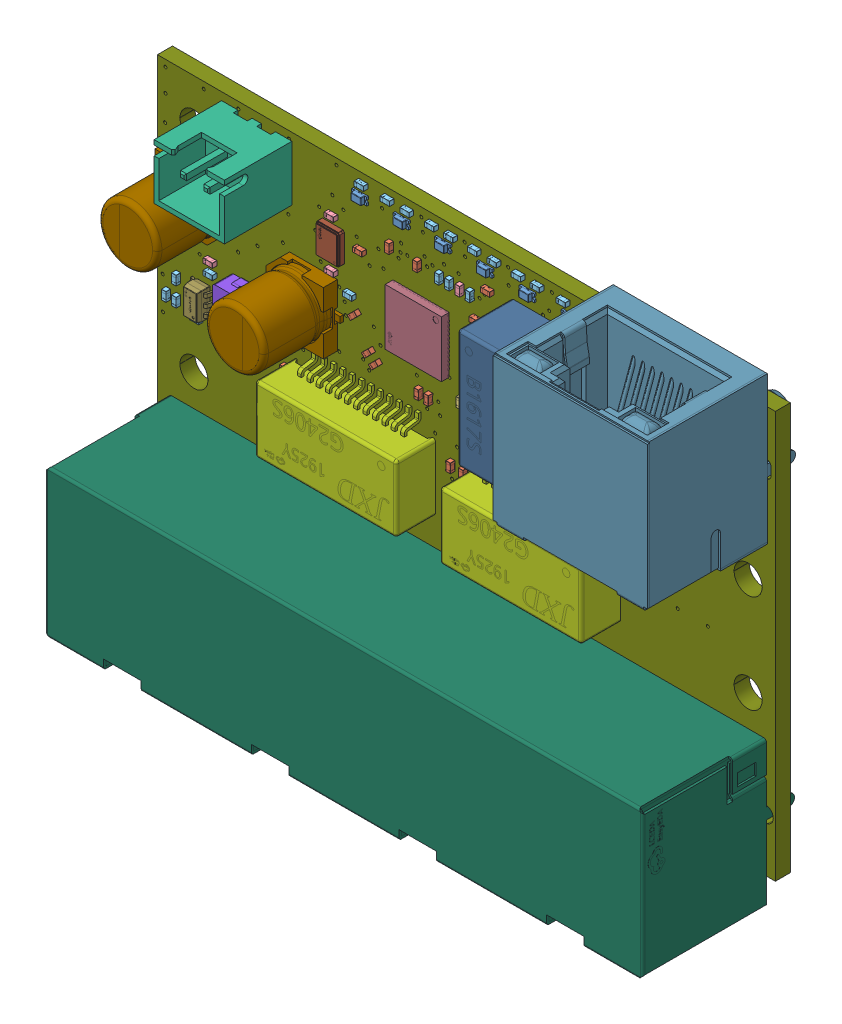
SolidWorks assembly 交换机, configuration 默认. Lengths in mm.
Overall size (65.92 49.68 16.5).
179 component instances, 16 part files, 0 mates.
Components (placement in the parent):
- LX-SWF502-2.step-1: LX-SWF502-2.step [Default] at (-129.5338 -11.9883 -6.5513) size (65.92 49.68 16.5)
  - RJEO-D19.step-1: RJEO-D19.step [Default] at (21.7657 41.0001 1.6) size (1.62 0.82 0.56)
    - LED0603N.step-1: LED0603N.step [Default] at origin size (1.62 0.82 0.56)
      - COMPOUND.step-1: COMPOUND.step [Default] at origin size (1.62 0.82 0.56)
  - RJEO-D2.step-1: RJEO-D2.step [Default] at (30.6411 41.0001 1.6) size (1.62 0.82 0.56)
    - LED0603N.step-1: LED0603N.step [Default] at origin size (1.62 0.82 0.56)
      - COMPOUND.step-1: COMPOUND.step [Default] at origin size (1.62 0.82 0.56)
  - RJEO-D20.step-1: RJEO-D20.step [Default] at (44.1334 41.0001 1.6) size (1.62 0.82 0.56)
    - LED0603N.step-1: LED0603N.step [Default] at origin size (1.62 0.82 0.56)
      - COMPOUND.step-1: COMPOUND.step [Default] at origin size (1.62 0.82 0.56)
  - RJEO-D21.step-1: RJEO-D21.step [Default] at (39.6501 41.0001 1.6) size (1.62 0.82 0.56)
    - LED0603N.step-1: LED0603N.step [Default] at origin size (1.62 0.82 0.56)
      - COMPOUND.step-1: COMPOUND.step [Default] at origin size (1.62 0.82 0.56)
  - RJEO-D22.step-1: RJEO-D22.step [Default] at (35.1271 41.0001 1.6) size (1.62 0.82 0.56)
    - LED0603N.step-1: LED0603N.step [Default] at origin size (1.62 0.82 0.56)
      - COMPOUND.step-1: COMPOUND.step [Default] at origin size (1.62 0.82 0.56)
  - RJEO-D1.step-1: RJEO-D1.step [Default] at (26.2147 41.0001 1.6) size (1.62 0.82 0.56)
    - LED0603N.step-1: LED0603N.step [Default] at origin size (1.62 0.82 0.56)
      - COMPOUND.step-1: COMPOUND.step [Default] at origin size (1.62 0.82 0.56)
  - RJEO-C10.step-1: RJEO-C10.step [Default] at (28.0001 37.4021 1.6) x (0 1 0) z (0 0 1) size (1 0.5 0.5)
    - 0402.step-1: 0402.step [Default] at origin size (1 0.5 0.5)
      - SOLID.step-1: SOLID.step [Default] at origin size (1 0.5 0.5)
  - RJEO-C11.step-1: RJEO-C11.step [Default] at (22.346 36.1431 1.6) x (-1 0 0) z (0 0 1) size (1 0.5 0.5)
    - 0402.step-1: 0402.step [Default] at origin size (1 0.5 0.5)
      - SOLID.step-1: SOLID.step [Default] at origin size (1 0.5 0.5)
  - RJEO-C13.step-1: RJEO-C13.step [Default] at (28.1391 26.6451 1.6) x (0 -1 0) z (0 0 1) size (1 0.5 0.5)
    - 0402.step-1: 0402.step [Default] at origin size (1 0.5 0.5)
      - SOLID.step-1: SOLID.step [Default] at origin size (1 0.5 0.5)
  - RJEO-C14.step-1: RJEO-C14.step [Default] at (32.6271 28.0611 1.6) x (0 -1 0) z (0 0 1) size (1 0.5 0.5)
    - 0402-1.step-1: 0402-1.step [Default] at origin size (1 0.5 0.5)
      - SOLID-0.step-1: SOLID-0.step [Default] at origin size (1 0.5 0.5)
  - RJEO-C15.step-1: RJEO-C15.step [Default] at (33.7611 35.9131 1.6) size (1 0.5 0.5)
    - 0402.step-1: 0402.step [Default] at origin size (1 0.5 0.5)
      - SOLID.step-1: SOLID.step [Default] at origin size (1 0.5 0.5)
  - RJEO-C16.step-1: RJEO-C16.step [Default] at (25.0001 37.5751 1.6) x (0 1 0) z (0 0 1) size (1 0.5 0.5)
    - 0402.step-1: 0402.step [Default] at origin size (1 0.5 0.5)
      - SOLID.step-1: SOLID.step [Default] at origin size (1 0.5 0.5)
  - RJEO-C17.step-1: RJEO-C17.step [Default] at (21.666 30.3191 1.6) x (-0.707107 -0.707107 0) z (0 0 1) size (1 0.5 0.5)
    - 0402.step-1: 0402.step [Default] at origin size (1 0.5 0.5)
      - SOLID.step-1: SOLID.step [Default] at origin size (1 0.5 0.5)
  - RJEO-C18.step-1: RJEO-C18.step [Default] at (23.917 26.8671 1.6) x (-0.707107 -0.707107 0) z (0 0 1) size (1 0.5 0.5)
    - 0402.step-1: 0402.step [Default] at origin size (1 0.5 0.5)
      - SOLID.step-1: SOLID.step [Default] at origin size (1 0.5 0.5)
  - RJEO-C19.step-1: RJEO-C19.step [Default] at (34.9891 39.2441 1.6) size (1 0.5 0.5)
    - 0402.step-1: 0402.step [Default] at origin size (1 0.5 0.5)
      - SOLID.step-1: SOLID.step [Default] at origin size (1 0.5 0.5)
  - RJEO-C2.step-1: RJEO-C2.step [Default] at (32.8971 20.6 1.6) x (0 1 0) z (0 0 1) size (1 0.5 0.5)
    - 0402.step-1: 0402.step [Default] at origin size (1 0.5 0.5)
      - SOLID.step-1: SOLID.step [Default] at origin size (1 0.5 0.5)
  - RJEO-C20.step-1: RJEO-C20.step [Default] at (31.5481 20.6 1.6) x (0 1 0) z (0 0 1) size (1 0.5 0.5)
    - 0402.step-1: 0402.step [Default] at origin size (1 0.5 0.5)
      - SOLID.step-1: SOLID.step [Default] at origin size (1 0.5 0.5)
  - RJEO-C25.step-1: RJEO-C25.step [Default] at (13.815 20.6 1.6) x (0 1 0) z (0 0 1) size (1 0.5 0.5)
    - 0402.step-1: 0402.step [Default] at origin size (1 0.5 0.5)
      - SOLID.step-1: SOLID.step [Default] at origin size (1 0.5 0.5)
  - RJEO-C37.step-1: RJEO-C37.step [Default] at (23.177 27.5921 1.6) x (-0.707107 -0.707107 0) z (0 0 1) size (1 0.5 0.5)
    - 0402.step-1: 0402.step [Default] at origin size (1 0.5 0.5)
      - SOLID.step-1: SOLID.step [Default] at origin size (1 0.5 0.5)
  - RJEO-C7.step-1: RJEO-C7.step [Default] at (34.7321 30.7291 1.6) x (0 -1 0) z (0 0 1) size (1 0.5 0.5)
    - 0402.step-1: 0402.step [Default] at origin size (1 0.5 0.5)
      - SOLID.step-1: SOLID.step [Default] at origin size (1 0.5 0.5)
  - RJEO-C8.step-1: RJEO-C8.step [Default] at (29.1961 26.6451 1.6) x (0 -1 0) z (0 0 1) size (1 0.5 0.5)
    - 0402.step-1: 0402.step [Default] at origin size (1 0.5 0.5)
      - SOLID.step-1: SOLID.step [Default] at origin size (1 0.5 0.5)
  - RJEO-C21.step-1: RJEO-C21.step [Default] at (5.908 27.1321 1.6) x (-1 0 0) z (0 0 1) size (1 0.5 0.5)
    - C0402.step-1: C0402.step [Default] at origin size (1 0.5 0.5)
      - SOLID-1.step-1: SOLID-1.step [Default] at origin size (1 0.5 0.5)
  - RJEO-C22.step-1: RJEO-C22.step [Default] at (6.552 21.19 1.6) size (1 0.5 0.5)
    - C0402.step-1: C0402.step [Default] at origin size (1 0.5 0.5)
      - SOLID-1.step-1: SOLID-1.step [Default] at origin size (1 0.5 0.5)
  - RJEO-C3.step-1: RJEO-C3.step [Default] at (32.5331 37.9101 1.6) x (0 1 0) z (0 0 1) size (1 0.5 0.5)
    - C0402.step-1: C0402.step [Default] at origin size (1 0.5 0.5)
      - SOLID-1.step-1: SOLID-1.step [Default] at origin size (1 0.5 0.5)
  - RJEO-C4.step-1: RJEO-C4.step [Default] at (18.817 32.7271 1.6) x (-1 0 0) z (0 0 1) size (1 0.5 0.5)
    - C0402.step-1: C0402.step [Default] at origin size (1 0.5 0.5)
      - SOLID-1.step-1: SOLID-1.step [Default] at origin size (1 0.5 0.5)
  - RJEO-C5.step-1: RJEO-C5.step [Default] at (18.81 37.8231 1.6) x (-1 0 0) z (0 0 1) size (1 0.5 0.5)
    - C0402.step-1: C0402.step [Default] at origin size (1 0.5 0.5)
      - SOLID-1.step-1: SOLID-1.step [Default] at origin size (1 0.5 0.5)
  - RJEO-C1.step-1: RJEO-C1.step [Default] at (51.3311 20.6 1.6) x (0 1 0) z (0 0 1) size (1 0.5 0.5)
    - 0402.step-1: 0402.step [Default] at origin size (1 0.5 0.5)
      - SOLID.step-1: SOLID.step [Default] at origin size (1 0.5 0.5)
  - RJEO-R11.step-1: RJEO-R11.step [Default] at (6.402 25.9921 1.6) x (-1 0 0) z (0 0 1) size (1 0.5 0.5)
    - 0402-2.step-1: 0402-2.step [Default] at origin size (1 0.5 0.5)
      - SOLID-2.step-1: SOLID-2.step [Default] at origin size (1 0.5 0.5)
  - RJEO-R12.step-1: RJEO-R12.step [Default] at (3.948 21.19 1.6) size (1 0.5 0.5)
    - 0402-2.step-1: 0402-2.step [Default] at origin size (1 0.5 0.5)
      - SOLID-2.step-1: SOLID-2.step [Default] at origin size (1 0.5 0.5)
  - RJEO-R13.step-1: RJEO-R13.step [Default] at (1.211 22.273 1.6) x (0 -1 0) z (0 0 1) size (1 0.5 0.5)
    - 0402-2.step-1: 0402-2.step [Default] at origin size (1 0.5 0.5)
      - SOLID-2.step-1: SOLID-2.step [Default] at origin size (1 0.5 0.5)
  - RJEO-R14.step-1: RJEO-R14.step [Default] at (2.295 24.326 1.6) x (0 -1 0) z (0 0 1) size (1 0.5 0.5)
    - 0402-2.step-1: 0402-2.step [Default] at origin size (1 0.5 0.5)
      - SOLID-2.step-1: SOLID-2.step [Default] at origin size (1 0.5 0.5)
  - RJEO-R15.step-1: RJEO-R15.step [Default] at (2.295 21.285 1.6) x (0 1 0) z (0 0 1) size (1 0.5 0.5)
    - 0402-2.step-1: 0402-2.step [Default] at origin size (1 0.5 0.5)
      - SOLID-2.step-1: SOLID-2.step [Default] at origin size (1 0.5 0.5)
  - RJEO-R2.step-1: RJEO-R2.step [Default] at (20.272 31.5191 1.6) size (1 0.5 0.5)
    - 0402-2.step-1: 0402-2.step [Default] at origin size (1 0.5 0.5)
      - SOLID-2.step-1: SOLID-2.step [Default] at origin size (1 0.5 0.5)
  - RJEO-R20.step-1: RJEO-R20.step [Default] at (26.4001 42.3001 1.6) size (1 0.5 0.5)
    - 0402-2.step-1: 0402-2.step [Default] at origin size (1 0.5 0.5)
      - SOLID-2.step-1: SOLID-2.step [Default] at origin size (1 0.5 0.5)
  - RJEO-R21.step-1: RJEO-R21.step [Default] at (31.0661 42.3001 1.6) size (1 0.5 0.5)
    - 0402-2.step-1: 0402-2.step [Default] at origin size (1 0.5 0.5)
      - SOLID-2.step-1: SOLID-2.step [Default] at origin size (1 0.5 0.5)
  - RJEO-R22.step-1: RJEO-R22.step [Default] at (35.6971 42.3001 1.6) size (1 0.5 0.5)
    - 0402-2.step-1: 0402-2.step [Default] at origin size (1 0.5 0.5)
      - SOLID-2.step-1: SOLID-2.step [Default] at origin size (1 0.5 0.5)
  - RJEO-R23.step-1: RJEO-R23.step [Default] at (40.2871 42.3001 1.6) size (1 0.5 0.5)
    - 0402-2.step-1: 0402-2.step [Default] at origin size (1 0.5 0.5)
      - SOLID-2.step-1: SOLID-2.step [Default] at origin size (1 0.5 0.5)
  - RJEO-R24.step-1: RJEO-R24.step [Default] at (45.0261 42.3001 1.6) size (1 0.5 0.5)
    - 0402-2.step-1: 0402-2.step [Default] at origin size (1 0.5 0.5)
      - SOLID-2.step-1: SOLID-2.step [Default] at origin size (1 0.5 0.5)
  - RJEO-R26.step-1: RJEO-R26.step [Default] at (21.524 42.3001 1.6) size (1 0.5 0.5)
    - 0402-2.step-1: 0402-2.step [Default] at origin size (1 0.5 0.5)
      - SOLID-2.step-1: SOLID-2.step [Default] at origin size (1 0.5 0.5)
  - RJEO-R3.step-1: RJEO-R3.step [Default] at (33.6221 38.4311 1.6) x (0 -1 0) z (0 0 1) size (1 0.5 0.5)
    - 0402-2.step-1: 0402-2.step [Default] at origin size (1 0.5 0.5)
      - SOLID-2.step-1: SOLID-2.step [Default] at origin size (1 0.5 0.5)
  - RJEO-R4.step-1: RJEO-R4.step [Default] at (30.3291 38.4071 1.6) x (0 -1 0) z (0 0 1) size (1 0.5 0.5)
    - 0402-2.step-1: 0402-2.step [Default] at origin size (1 0.5 0.5)
      - SOLID-2.step-1: SOLID-2.step [Default] at origin size (1 0.5 0.5)
  - RJEO-R5.step-1: RJEO-R5.step [Default] at (44.0581 42.3001 1.6) x (-1 0 0) z (0 0 1) size (1 0.5 0.5)
    - 0402-2.step-1: 0402-2.step [Default] at origin size (1 0.5 0.5)
      - SOLID-2.step-1: SOLID-2.step [Default] at origin size (1 0.5 0.5)
  - RJEO-R6.step-1: RJEO-R6.step [Default] at (39.2791 42.3001 1.6) x (-1 0 0) z (0 0 1) size (1 0.5 0.5)
    - 0402-2.step-1: 0402-2.step [Default] at origin size (1 0.5 0.5)
      - SOLID-2.step-1: SOLID-2.step [Default] at origin size (1 0.5 0.5)
  - RJEO-R7.step-1: RJEO-R7.step [Default] at (34.6091 42.3001 1.6) x (-1 0 0) z (0 0 1) size (1 0.5 0.5)
    - 0402-2.step-1: 0402-2.step [Default] at origin size (1 0.5 0.5)
      - SOLID-2.step-1: SOLID-2.step [Default] at origin size (1 0.5 0.5)
  - RJEO-R8.step-1: RJEO-R8.step [Default] at (30.0421 42.3001 1.6) x (-1 0 0) z (0 0 1) size (1 0.5 0.5)
    - 0402-2.step-1: 0402-2.step [Default] at origin size (1 0.5 0.5)
      - SOLID-2.step-1: SOLID-2.step [Default] at origin size (1 0.5 0.5)
  - RJEO-R9.step-1: RJEO-R9.step [Default] at (25.3031 42.3001 1.6) x (-1 0 0) z (0 0 1) size (1 0.5 0.5)
    - 0402-2.step-1: 0402-2.step [Default] at origin size (1 0.5 0.5)
      - SOLID-2.step-1: SOLID-2.step [Default] at origin size (1 0.5 0.5)
  - RJEO-R1.step-1: RJEO-R1.step [Default] at (31.4191 37.4141 1.6) x (0 1 0) z (0 0 1) size (1 0.5 0.5)
    - 0402-2.step-1: 0402-2.step [Default] at origin size (1 0.5 0.5)
      - SOLID-2.step-1: SOLID-2.step [Default] at origin size (1 0.5 0.5)
  - RJEO-JP1.step-1: RJEO-JP1.step [Default] at (12.001 40.0001 1.6) x (-1 0 0) z (0 0 1) size (7.5 5.9 10.6)
    - SIP2.step-1: SIP2.step [Default] at origin size (7.5 5.9 10.6)
      - COMPOUND-3.step-1: COMPOUND-3.step [Default] at origin size (7.5 5.9 10.6)
  - RJEO-DXFRM3.step-1: RJEO-DXFRM3.step [Default] at (21.989 19.3 1.6) x (-1 0 0) z (0 0 1) size (15.1 10 4.5)
    - NS892407B.step-1: NS892407B.step [Default] at origin size (15.1 10 4.5)
      - COMPOUND-4.step-1: COMPOUND-4.step [Default] at origin size (15.1 10 4.5)
  - RJEO-DXFRM1.step-1: RJEO-DXFRM1.step [Default] at (41.7141 19.3 1.6) x (-1 0 0) z (0 0 1) size (15.1 10 4.5)
    - NS892407B.step-1: NS892407B.step [Default] at origin size (15.1 10 4.5)
      - COMPOUND-4.step-1: COMPOUND-4.step [Default] at origin size (15.1 10 4.5)
  - RJEO-L2.step-1: RJEO-L2.step [Default] at (10.114 25.031 1.6) x (0 -1 0) z (0 0 1) size (4.4 4.2 2.1)
    - L10A.step-1: L10A.step [Default] at origin size (4.4 4.2 2.1)
      - SOLID-5.step-1: SOLID-5.step [Default] at origin size (4.4 4.2 2.1)
  - RJEO-TC4.step-1: RJEO-TC4.step [Default] at (4.629 32.6291 1.6) x (0 -1 0) z (0 0 1) size (6.6 7.8 7.75)
    - CAP-E-SMD-D6.3.step-1: CAP-E-SMD-D6.3.step [Default] at origin size (6.6 7.8 7.75)
      - SOLID-6.step-1: SOLID-6.step [Default] at origin size (6.6 7.8 7.75)
  - RJEO-TC1.step-1: RJEO-TC1.step [Default] at (16 28.8001 1.6) x (0 1 0) z (0 0 1) size (6.6 7.8 7.75)
    - CAP-E-SMD-D6.3.step-1: CAP-E-SMD-D6.3.step [Default] at origin size (6.6 7.8 7.75)
      - SOLID-6.step-1: SOLID-6.step [Default] at origin size (6.6 7.8 7.75)
  - RJEO-TRS1.step-1: RJEO-TRS1.step [Default] at (41.5201 33.5001 1.6) x (0 -1 0) z (0 0 1) size (12.7 9.5 5.95)
    - RJ45-8PIN.step-1: RJ45-8PIN.step [Default] at origin size (12.7 9.5 5.95)
      - COMPOUND-7.step-1: COMPOUND-7.step [Default] at origin size (12.7 9.5 5.95)
  - RJEO-Y6.step-1: RJEO-Y6.step [Default] at (18.772 35.3521 1.6) x (0 1 0) z (0 0 1) size (3.2 2.5 0.72)
    - SM091.step-1: SM091.step [Default] at origin size (3.2 2.5 0.72)
      - SOLID-8.step-1: SOLID-8.step [Default] at origin size (3.2 2.5 0.72)
  - RJEO-U1.step-1: RJEO-U1.step [Default] at (6.457 22.482 1.6) x (0 1 0) z (0 0 1) size (2.88 2.79 1.64)
    - SOT23-6.step-1: SOT23-6.step [Default] at origin size (2.88 2.79 1.64)
      - COMPOUND-9.step-1: COMPOUND-9.step [Default] at origin size (2.88 2.79 1.64)
  - RJEO-U2.step-1: RJEO-U2.step [Default] at (28.0001 32.0001 1.6) x (-1 0 0) z (0 0 1) size (6 6 0.85)
    - QFN48_04_EPAD.step-1: QFN48_04_EPAD.step [Default] at origin size (6 6 0.85)
      - COMPOUND-10.step-1: COMPOUND-10.step [Default] at origin size (6 6 0.85)
  - RJEO-H6.step-1: RJEO-H6.step [Default] at (56.8961 40.8691 1.6) x (-1 0 0) z (0 0 1) size (16.45 16.05 15.8)
    - RJ45-1X1-B.step-1: RJ45-1X1-B.step [Default] at origin size (16.45 16.05 15.8)
      - COMPOUND-11.step-1: COMPOUND-11.step [Default] at origin size (16.45 16.05 15.8)
  - RJEO-H7.step-1: RJEO-H7.step [Default] at (33.1521 2.093 1.6) size (63.76 15.76 16.2)
    - RJ45-1X4-B.step-1: RJ45-1X4-B.step [Default] at origin size (63.76 15.76 16.2)
      - COMPOUND-12.step-1: COMPOUND-12.step [Default] at origin size (63.76 15.76 16.2)
  - Board.step-1: Board.step [Default] at origin size (65.92 43.41 1.6)
